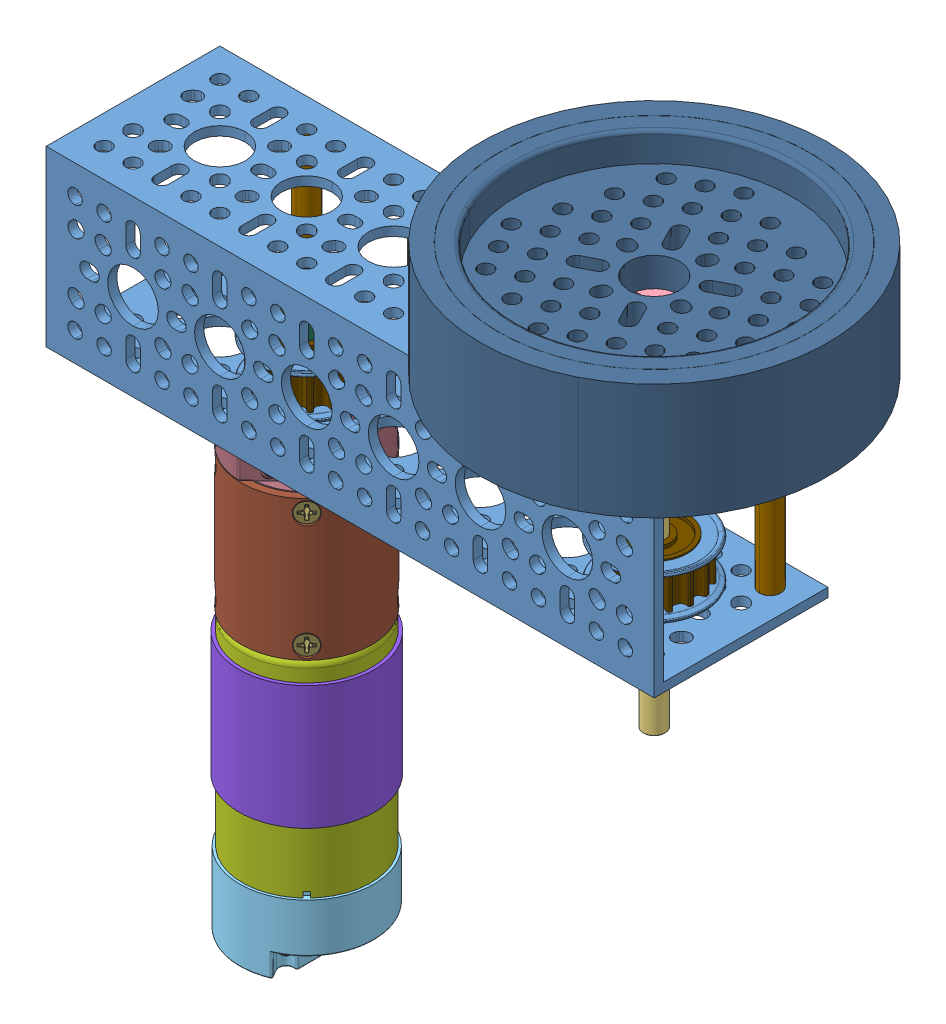
SolidWorks assembly motorisationGauche, configuration Défaut. Lengths in mm.
Overall size (208.53 212.25 129.07).
69 component instances, 28 part files, 28 mates.
Components (placement in the parent):
- 1120-0006-0168 channel-1: 1120-0006-0168 channel [Défaut] at (77.3616 4.0114 -146.5) x (0 1 0) z (0 0 1) size (48 168 48)
- 5202-2402-0051 moteur-1: 5202-2402-0051 moteur [Défaut] at (-76.7557 -130.424 -149.55) x (-0.707107 0 0.707107) z (-0.707107 0 -0.707107) size (52.36 150.75 52.36)
  - 5202-2402-0051.step-1: 5202-2402-0051.step [Défaut] at origin size (52.36 150.75 52.36)
    - 5000-0002-0001.step-1: 5000-0002-0001.step [Défaut] at origin size (52.36 88.75 52.36)
      - 5000-0002-0001 encoder cap.step-1: 5000-0002-0001 encoder cap.step [Défaut] x (0 1 0) z (0 0 1) size (22.84 52.33 52.33)
        - JST-XH-4POS-VERT (1).step-1: JST-XH-4POS-VERT (1).step [Défaut] at (2.8 12.25 -75.95) x (1 0 0) z (0 0 -1) size (10.4 12.83 12.83)
          - Plastic (1).step-1: Plastic (1).step [Défaut] at (-6.1146 -33.6358 -52.1967) x (0 0.707107 0.707107) z (-1 0 0) size (12.4 5.75 7)
          - Pin (1).step-1: Pin (1).step [Défaut] at (-7.7146 -29.3225 -51.2067) x (0 0.707107 0.707107) z (-1 0 0) size (0.64 0.64 10)
          - Pin (1).step-2: Pin (1).step [Défaut] at (-7.7146 -34.6258 -56.51) x (0 0.707107 0.707107) z (-1 0 0) size (0.64 0.64 10)
          - Pin (1).step-3: Pin (1).step [Défaut] at (-7.7146 -32.858 -54.7423) x (0 0.707107 0.707107) z (-1 0 0) size (0.64 0.64 10)
          - Pin (1).step-4: Pin (1).step [Défaut] at (-7.7146 -31.0902 -52.9745) x (0 0.707107 0.707107) z (-1 0 0) size (0.64 0.64 10)
        - screw.step-1: screw.step [Défaut] at (-41.264 -8.1646 3.9905) x (0.882398 0 0.470504) z (0 -1 0) size (8.86 7.85 4.95)
          - 99461A915_Phillips Rounded Head Thread-Forming Screws (1).step-1: 99461A915_Phillips Rounded Head Thread-Forming Screws (1).step [Défaut] at (27.264 -14.6475 -49.347) x (-0.332697 -0.623949 0.707107) z (-0.882398 0.470504 0) size (3.5 3.5 7.4)
        - screw_1.step-1: screw_1.step [Défaut] at (-14.4172 7.3354 3.9905) x (0.882398 0 0.470504) z (0 -1 0) size (8.86 7.85 4.95)
          - 99461A915_Phillips Rounded Head Thread-Forming Screws (1).step-1: 99461A915_Phillips Rounded Head Thread-Forming Screws (1).step [Défaut] at (-10.5142 -28.4382 -25.8237) x (-0.332697 -0.623949 0.707107) z (-0.882398 0.470504 0) size (3.5 3.5 7.4)
        - endcap.step-1: endcap.step [Défaut] at (72.6354 37.1707 -11.0784) x (0 -0.707107 -0.707107) z (1 0 0) size (37 37 21.84)
        - base.step-1: base.step [Défaut] at (-55.8646 37.1707 -11.0784) x (0 -0.707107 -0.707107) z (-1 0 0) size (34.96 34.31 1)
      - 5000-0002-0001 body.step-1: 5000-0002-0001 body.step [Défaut] at (-37.1707 3.4854 -11.0784) size (35.61 61.8 35.61)
      - 5000-0002-0001 motor shield.step-1: 5000-0002-0001 motor shield.step [Défaut] at (-37.1707 54.6354 -11.0784) x (0.808104 0 -0.58904) z (0 -1 0) size (37.5 37.27 34.15)
      - 5000-0002-0001 motor shaft.step-1: 5000-0002-0001 motor shaft.step [Défaut] at (-37.1707 59.4854 -11.0784) size (3.14 12.45 3.14)
    - 5102-0024-0051.step-1: 5102-0024-0051.step [Défaut] at origin size (36 76.68 35.98)
      - 5102 Gearbox Base.step-1: 5102 Gearbox Base.step [Défaut] at (-37.1707 60.1354 -11.0784) size (31.91 5.69 31.91)
      - 5102 Gearbox Barrel (3 stage, simple)_Gear Blank.step-1: 5102 Gearbox Barrel (3 stage, simple)_Gear Blank.step [Défaut] at (-37.1707 111.8354 -11.0784) x (1 0 0) z (0 -1 0) size (35.98 35.98 38.7)
      - 5102 Gearbox Barrel Screw (M3 x 8mm length Flat Head)_92010A118.step-1: 5102 Gearbox Barrel Screw (M3 x 8mm length Flat Head)_92010A118.step [Défaut] at (-37.1707 63.6354 5.0046) x (0.002439 -0.999997 0) z (0 0 1) size (5.46 5.46 8)
      - 5102 Gearbox Face.step-1: 5102 Gearbox Face.step [Défaut] at (-37.1707 93.3354 -11.0784) size (36 17.1 31.91)
      - 5102 Gearbox Bearing.step-1: 5102 Gearbox Bearing.step [Défaut] at (-37.1707 101.4354 -11.0784) size (17 5 17)
      - 5102 Gearbox Shaft (23.5mm Length, Simple).step-1: 5102 Gearbox Shaft (23.5mm Length, Simple).step [Défaut] at (-37.1707 89.9754 -11.0784) x (0.894773 0 -0.44652) z (0.44652 0 0.894773) size (8.97 40.6 8.97)
      - 5102 Gearbox Snap Ring.step-1: 5102 Gearbox Snap Ring.step [Défaut] at (-37.1707 106.5104 -11.0784) x (0 1 0) z (0 0 1) size (0.85 13.06 10.66)
      - 5102 Gearbox Barrel Screw (M3 x 8mm length Flat Head)_92010A118.step-2: 5102 Gearbox Barrel Screw (M3 x 8mm length Flat Head)_92010A118.step [Défaut] at (-37.1707 95.3354 5.0046) x (-0.002439 -0.999997 0) z (0 0 1) size (5.46 5.46 8)
      - 5102 Gearbox Barrel Screw (M3 x 8mm length Flat Head)_92010A118.step-3: 5102 Gearbox Barrel Screw (M3 x 8mm length Flat Head)_92010A118.step [Défaut] at (-21.0877 63.6354 -11.0784) x (0 -0.999997 -0.002439) z (1 0 0) size (5.46 5.46 8)
      - 5102 Gearbox Barrel Screw (M3 x 8mm length Flat Head)_92010A118.step-4: 5102 Gearbox Barrel Screw (M3 x 8mm length Flat Head)_92010A118.step [Défaut] at (-37.1707 63.6354 -27.1614) x (-0.002439 -0.999997 0) z (0 0 -1) size (5.46 5.46 8)
      - 5102 Gearbox Barrel Screw (M3 x 8mm length Flat Head)_92010A118.step-5: 5102 Gearbox Barrel Screw (M3 x 8mm length Flat Head)_92010A118.step [Défaut] at (-53.2537 63.6354 -11.0784) x (0 -0.999997 0.002439) z (-1 0 0) size (5.46 5.46 8)
      - 5102 Gearbox Barrel Screw (M3 x 8mm length Flat Head)_92010A118.step-6: 5102 Gearbox Barrel Screw (M3 x 8mm length Flat Head)_92010A118.step [Défaut] at (-21.0877 95.3354 -11.0784) x (0 -0.999997 0.002439) z (1 0 0) size (5.46 5.46 8)
      - 5102 Gearbox Barrel Screw (M3 x 8mm length Flat Head)_92010A118.step-7: 5102 Gearbox Barrel Screw (M3 x 8mm length Flat Head)_92010A118.step [Défaut] at (-37.1707 95.3354 -27.1614) x (0.002439 -0.999997 0) z (0 0 -1) size (5.46 5.46 8)
      - 5102 Gearbox Barrel Screw (M3 x 8mm length Flat Head)_92010A118.step-8: 5102 Gearbox Barrel Screw (M3 x 8mm length Flat Head)_92010A118.step [Défaut] at (-53.2537 95.3354 -11.0784) x (0 -0.999997 -0.002439) z (-1 0 0) size (5.46 5.46 8)
      - 5102 Gearbox Bearing.step-2: 5102 Gearbox Bearing.step [Défaut] at (-37.1707 93.3354 -11.0784) size (17 5 17)
      - 5102 Gearbox Base Mounting Screw M3 x 5mm length SHCS)_91290A110.step-1: 5102 Gearbox Base Mounting Screw M3 x 5mm length SHCS)_91290A110.step [Défaut] at (-46.0096 57.2554 -2.2396) x (0.056382 0 0.998409) z (0 -1 0) size (5.5 5.5 8)
      - 5102 Gearbox Base Mounting Screw M3 x 5mm length SHCS)_91290A110.step-2: 5102 Gearbox Base Mounting Screw M3 x 5mm length SHCS)_91290A110.step [Défaut] at (-28.3319 57.2554 -2.2396) x (0.998409 0 -0.056382) z (0 -1 0) size (5.5 5.5 8)
      - 5102 Gearbox Base Mounting Screw M3 x 5mm length SHCS)_91290A110.step-3: 5102 Gearbox Base Mounting Screw M3 x 5mm length SHCS)_91290A110.step [Défaut] at (-28.3319 57.2554 -19.9173) x (-0.056382 0 -0.998409) z (0 -1 0) size (5.5 5.5 8)
      - 5102 Gearbox Base Mounting Screw M3 x 5mm length SHCS)_91290A110.step-4: 5102 Gearbox Base Mounting Screw M3 x 5mm length SHCS)_91290A110.step [Défaut] at (-46.0096 57.2554 -19.9173) x (-0.998409 0 0.056382) z (0 -1 0) size (5.5 5.5 8)
- 3417-1006-0016 assembly pulley-2: 3417-1006-0016 assembly pulley [Défaut] at (75.6511 44.9793 -178.9497) x (0 1 0) z (-0.665264 0 0.746608) size (12.01 27.98 27.98)
  - 3417-1006-0016 assembly.STEP-1: 3417-1006-0016 assembly.STEP [Défaut] at origin size (12.01 27.98 27.98)
    - 3417-1006-0016 body.STEP-1: 3417-1006-0016 body.STEP [Défaut] at (-62.7232 -4.1348 4.7756) size (12 23.97 23.97)
    - 3417-1006-0016 ring.STEP-1: 3417-1006-0016 ring.STEP [Défaut] at (-50.8429 9.3571 23.0035) x (0 -1 0) z (0 0 1) size (27.98 1.38 27.98)
    - 3417-1006-0016 ring.STEP-2: 3417-1006-0016 ring.STEP [Défaut] at (-60.0929 9.3571 23.0035) x (0 -1 0) z (0 0 -1) size (27.98 1.38 27.98)
    - 2806-0005-0006_91390A118.STEP-1: 2806-0005-0006_91390A118.STEP [Défaut] at (-55.4679 9.3571 17.1119) x (-0.607877 0.794031 0) z (0 0 -1) size (5.01 5.01 6.01)
- 2101-0006-0100 essieuCourt-1: 2101-0006-0100 essieuCourt [Défaut] at (53.3616 -50.9886 -168) x (0.958598 0 0.284763) z (-0.284763 0 0.958598) size (6 100 5.5)
- 1309-0016-1006 assembly-1: 1309-0016-1006 assembly [Défaut] at (44.1811 53.785 -183.7277) x (-0.476473 0 -0.879189) z (0 -1 0) size (28.36 32 10.95)
  - 1309-0016-1006 assembly.STEP-1: 1309-0016-1006 assembly.STEP [Défaut] at origin size (28.36 32 10.95)
    - 1309-0016-1006.STEP-1: 1309-0016-1006.STEP [Défaut] at (-18.2019 0.5776 8.7736) size (25.38 32 10)
    - 2800-0004-0014_90128A207.STEP-1: 2800-0004-0014_90128A207.STEP [Défaut] at (-16.149 11.6963 8.7736) x (0.5 -0.5 -0.707107) z (0.707107 0.707107 0) size (7 7 18.01)
    - 2800-0004-0014_90128A207.STEP-2: 2800-0004-0014_90128A207.STEP [Défaut] at (-20.2547 -10.5411 8.7736) x (-0.5 0.5 -0.707107) z (-0.707107 -0.707107 0) size (7 7 18.01)
- 1611-0514-0006-1: 1611-0514-0006 [Défaut] at (53.3616 -21.4886 -168) x (0.99842 0 -0.056195) z (0.056195 0 0.99842) size (15 5 15)
- 1611-0514-0006-2: 1611-0514-0006 [Défaut] at (53.3616 29.5114 -168) x (-1 0 0) z (0 0 1) size (15 5 15)
- 2910-0919-0006 assembly collet-2: 2910-0919-0006 assembly collet [Défaut] at (39.6619 20.0318 -135.4945) x (-0.7789 0 0.627148) z (-0.627148 0 -0.7789) size (19 9.89 19.83)
  - 2910-0919-0006 assembly.STEP-1: 2910-0919-0006 assembly.STEP [Défaut] at origin size (19 9.89 19.83)
    - 2910-0919-0006.STEP-1: 2910-0919-0006.STEP [Défaut] at (-31.0565 -0.5204 16.7268) size (19 9.5 18.97)
    - 2800-0004-0010_90128A207.STEP-1: 2800-0004-0010_90128A207.STEP [Défaut] at (-24.2865 -0.5204 11.2868) x (0 -0.807243 -0.59022) z (1 0 0) size (7 7 14.01)
- 1501-0006-0430 renfort-1: 1501-0006-0430 renfort [Défaut] at (69.3616 4.0114 -184) size (5.95 43.01 5.95)
- 1501-0006-0430 renfort-2: 1501-0006-0430 renfort [Défaut] at (37.3616 4.0114 -184) size (5.95 43.01 5.95)
- 1501-0006-0430 renfort-3: 1501-0006-0430 renfort [Défaut] at (-58.6384 4.0114 -184) size (5.95 43.01 5.95)
- 1501-0006-0430 renfort-4: 1501-0006-0430 renfort [Défaut] at (-26.6384 4.0114 -184) size (5.95 43.01 5.95)
- 3417-1006-0016 assembly pulley-3: 3417-1006-0016 assembly pulley [Défaut] at (-18.6478 44.9793 -174.4162) x (0 1 0) z (-0.797499 0 0.60332) size (12.01 27.98 27.98)
  - 3417-1006-0016 assembly.STEP-1: 3417-1006-0016 assembly.STEP [Défaut] at origin size (12.01 27.98 27.98)
    - 3417-1006-0016 body.STEP-1: 3417-1006-0016 body.STEP [Défaut] at (-62.7232 -4.1348 4.7756) size (12 23.97 23.97)
    - 3417-1006-0016 ring.STEP-1: 3417-1006-0016 ring.STEP [Défaut] at (-50.8429 9.3571 23.0035) x (0 -1 0) z (0 0 1) size (27.98 1.38 27.98)
    - 3417-1006-0016 ring.STEP-2: 3417-1006-0016 ring.STEP [Défaut] at (-60.0929 9.3571 23.0035) x (0 -1 0) z (0 0 -1) size (27.98 1.38 27.98)
    - 2806-0005-0006_91390A118.STEP-1: 2806-0005-0006_91390A118.STEP [Défaut] at (-55.4679 9.3571 17.1119) x (-0.607877 0.794031 0) z (0 0 -1) size (5.01 5.01 6.01)
- 3601-0014-0096 part-1: 3601-0014-0096 part [Défaut] at (53.3616 33.0114 -168) x (0.891556 0 -0.452911) z (0 -1 0) size (96 96 32)
Mates (geometry in assembly coordinates):
- Coaxiale22: concentric: cylinder of 5202-2402-0051 moteur-1/5202-2402-0051.step-1/5102-0024-0051.step-1/5102 Gearbox Shaft (23.5mm Length, Simple).step-1 through (-42.6384 -21.9886 -168) axis (0 1 0) radius 3; cylinder of 1120-0006-0168 channel-1 through (-42.6384 -9.9886 -168) axis (0 -1 0) radius 7
- Coïncidente26: coincident: plane of 1120-0006-0168 channel-1 through (-90.6384 -19.9886 -192) normal (0 -1 0); plane of 5202-2402-0051 moteur-1/5202-2402-0051.step-1/5102-0024-0051.step-1/5102 Gearbox Face.step-1 through (-42.6384 -19.9886 -168) normal (0 1 0)
- Coïncidente28: coincident: plane of 1120-0006-0168 channel-1 through (-90.6384 25.5114 -146.5) normal (0 -1 0); plane of 1501-0006-0430 renfort-4 through (-26.6384 25.5114 -184) normal (0 1 0)
- Coaxiale23: concentric: cylinder of 1501-0006-0430 renfort-4 through (-26.6384 25.5114 -184) axis (0 -1 0) radius 2.975; circle of 1120-0006-0168 channel-1
- Coïncidente29: coincident: plane of 1120-0006-0168 channel-1 through (-90.6384 25.5114 -146.5) normal (0 -1 0); plane of 1501-0006-0430 renfort-3 through (-58.6384 25.5114 -184) normal (0 1 0)
- Coaxiale24: concentric: cylinder of 1501-0006-0430 renfort-3 through (-58.6384 25.5114 -184) axis (0 -1 0) radius 2.975; cylinder of 1120-0006-0168 channel-1 through (-58.6384 18.0114 -184) axis (0 1 0) radius 2
- Coaxiale31: concentric: cylinder of 5202-2402-0051 moteur-1/5202-2402-0051.step-1/5102-0024-0051.step-1/5102 Gearbox Shaft (23.5mm Length, Simple).step-1 through (-42.6384 -21.9886 -168) axis (0 1 0) radius 3; cylinder of 3417-1006-0016 assembly pulley-3/3417-1006-0016 assembly.STEP-1/3417-1006-0016 body.STEP-1 through (-42.6384 -27.1188 -168) axis (0 1 0) radius 3
- Coaxiale32: concentric: cylinder of 2101-0006-0100 essieuCourt-1 through (53.3616 49.0114 -168) axis (0 -1 0) radius 3; cylinder of 1611-0514-0006-1 through (53.3616 -21.4886 -168) axis (0 1 0) radius 3
- Coaxiale33: concentric: cylinder of 2101-0006-0100 essieuCourt-1 through (53.3616 49.0114 -168) axis (0 -1 0) radius 3; cylinder of 1611-0514-0006-2 through (53.3616 29.5114 -168) axis (0 -1 0) radius 3
- Coaxiale34: concentric: cylinder of 2101-0006-0100 essieuCourt-1 through (53.3616 49.0114 -168) axis (0 -1 0) radius 3; cylinder of 2910-0919-0006 assembly collet-2/2910-0919-0006 assembly.STEP-1/2910-0919-0006.STEP-1 through (53.3616 24.0114 -168) axis (0 -1 0) radius 3
- Coaxiale35: concentric: cylinder of 3417-1006-0016 assembly pulley-2/3417-1006-0016 assembly.STEP-1/3417-1006-0016 body.STEP-1 through (53.3616 -27.1188 -168) axis (0 1 0) radius 3; cylinder of 2101-0006-0100 essieuCourt-1 through (53.3616 49.0114 -168) axis (0 -1 0) radius 3
- Coïncidente38: coincident: plane of 1611-0514-0006-2 through (53.3616 24.5114 -168) normal (0 -1 0); plane of 2910-0919-0006 assembly collet-2/2910-0919-0006 assembly.STEP-1/2910-0919-0006.STEP-1 through (53.3616 24.5114 -168) normal (0 1 0)
- Coïncidente39: coincident: plane of 3417-1006-0016 assembly pulley-2/3417-1006-0016 assembly.STEP-1/3417-1006-0016 body.STEP-1 through (53.3616 -16.4886 -168) normal (0 -1 0); plane of 1611-0514-0006-1 through (53.3616 -16.4886 -168) normal (0 1 0)
- Coaxiale39: concentric: cylinder of 1120-0006-0168 channel-1 through (53.3616 18.0114 -168) axis (0 1 0) radius 7; cylinder of 2101-0006-0100 essieuCourt-1 through (53.3616 49.0114 -168) axis (0 -1 0) radius 3
- Coïncidente42: coincident: plane of 1120-0006-0168 channel-1 through (-90.6384 25.5114 -146.5) normal (0 -1 0); plane of 1611-0514-0006-2 through (53.3616 25.5114 -168) normal (0 1 0)
- Coïncidente43: coincident: plane of 1120-0006-0168 channel-1 through (-90.6384 -17.4886 -146.5) normal (0 1 0); plane of 1611-0514-0006-1 through (53.3616 -17.4886 -168) normal (0 -1 0)
- Coïncidente45: coincident: plane of 3417-1006-0016 assembly pulley-2/3417-1006-0016 assembly.STEP-1/3417-1006-0016 body.STEP-1 through (41.7747 -4.4886 -169.857) normal (0 1 0); plane of 3417-1006-0016 assembly pulley-3/3417-1006-0016 assembly.STEP-1/3417-1006-0016 body.STEP-1 through (-53.6447 -4.4886 -172.0701) normal (0 1 0)
- Coïncidente46: coincident: plane of 1120-0006-0168 channel-1 through (-90.6384 -17.4886 -146.5) normal (0 1 0); plane of 1501-0006-0430 renfort-2 through (37.3616 -17.4886 -184) normal (0 -1 0)
- Coaxiale40: concentric: cylinder of 1120-0006-0168 channel-1 through (37.3616 -9.9886 -184) axis (0 -1 0) radius 2; cylinder of 1501-0006-0430 renfort-2 through (37.3616 25.5114 -184) axis (0 -1 0) radius 2.975
- Coïncidente47: coincident: plane of 1120-0006-0168 channel-1 through (-90.6384 -17.4886 -146.5) normal (0 1 0); plane of 1501-0006-0430 renfort-1 through (69.3616 -17.4886 -184) normal (0 -1 0)
- Coaxiale41: concentric: cylinder of 1120-0006-0168 channel-1 through (69.3616 -9.9886 -184) axis (0 -1 0) radius 2; cylinder of 1501-0006-0430 renfort-1 through (69.3616 25.5114 -184) axis (0 -1 0) radius 2.975
- Coaxiale42: concentric: cylinder of 2101-0006-0100 essieuCourt-1 through (53.3616 49.0114 -168) axis (0 -1 0) radius 3; cylinder of 3601-0014-0096 part-1 through (53.3616 33.0114 -168) axis (0 1 0) radius 7
- Parallèle1: parallel: plane of 2101-0006-0100 essieuCourt-1 through (54.0735 49.0114 -170.3965) normal (0.284763 0 -0.958598); plane of 1309-0016-1006 assembly-1/1309-0016-1006 assembly.STEP-1/1309-0016-1006.STEP-1 through (54.0678 49.2619 -170.3773) normal (-0.284763 0 0.958598)
- Coaxiale43: concentric: cylinder of 2101-0006-0100 essieuCourt-1 through (53.3616 49.0114 -168) axis (0 -1 0) radius 3; cylinder of 1309-0016-1006 assembly-1/1309-0016-1006 assembly.STEP-1/1309-0016-1006.STEP-1 through (53.3616 49.2619 -168) axis (0 -1 0) radius 3
- Coïncidente49: coincident: plane of 2101-0006-0100 essieuCourt-1 through (53.3616 49.0114 -168) normal (0 1 0); plane of 1309-0016-1006 assembly-1/1309-0016-1006 assembly.STEP-1/1309-0016-1006.STEP-1 through (53.3616 49.0114 -168) normal (0 1 0)
- Coïncidente50: coincident: plane of 1309-0016-1006 assembly-1/1309-0016-1006 assembly.STEP-1/1309-0016-1006.STEP-1 through (53.3616 49.0114 -168) normal (0 1 0); plane of 3601-0014-0096 part-1 through (53.3616 49.0114 -168) normal (0 -1 0)
- Distance1: distance = 5 mm: plane of 3601-0014-0096 part-1 through (53.3616 33.0114 -168) normal (0 -1 0); plane of 1120-0006-0168 channel-1 through (-90.6384 28.0114 -192) normal (0 1 0)
- Coaxiale44: concentric: circle of 1120-0006-0168 channel-1; circle of 5202-2402-0051 moteur-1/5202-2402-0051.step-1/5102-0024-0051.step-1/5102 Gearbox Face.step-1
